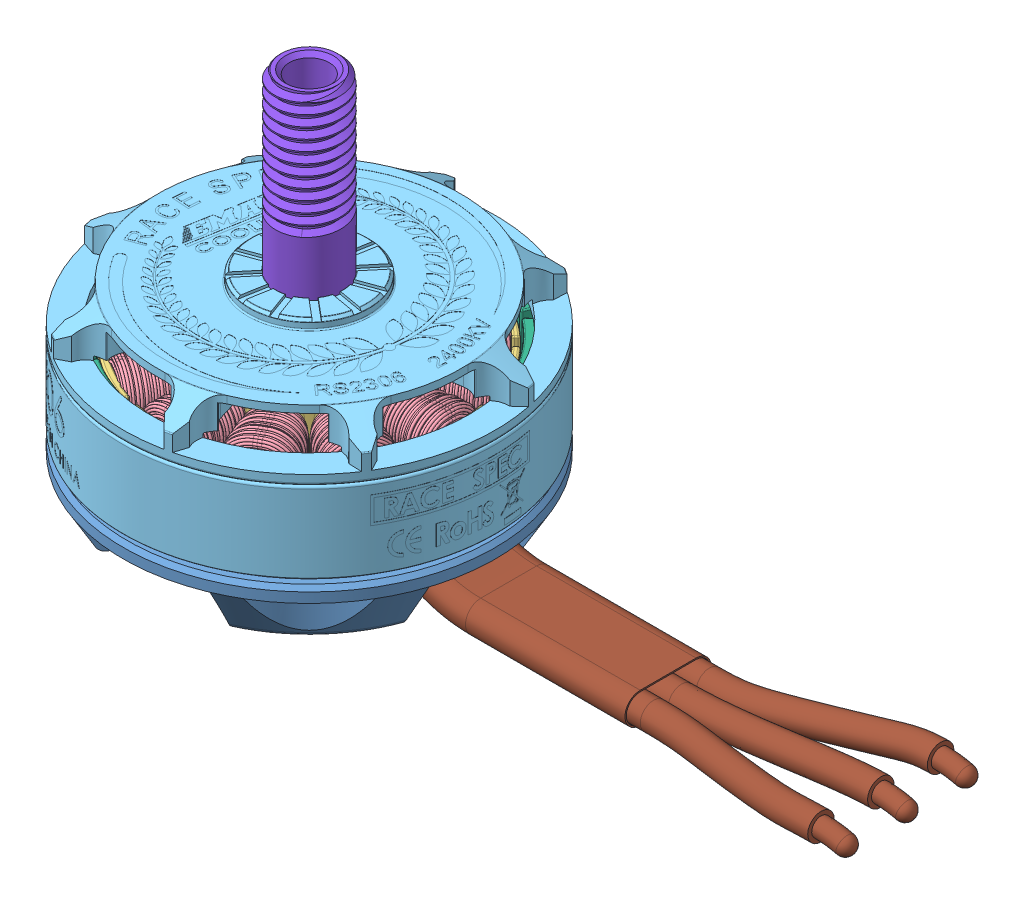
SolidWorks assembly EMAX RS2306, configuration Predeterminado. Lengths in mm.
Overall size (61.73 30.3 32.43).
25 component instances, 11 part files, 14 mates.
Components (placement in the parent):
- STATOR RS2306-1: STATOR RS2306 [Predeterminado] at origin size (28 11.98 28)
  - STATOR RS2306-1: STATOR RS2306 [Predeterminado] at origin size (28 10.77 28)
  - BEARING-1: BEARING [Predeterminado] at (0 2.25 0) x (1 0 0) z (0 1 0) size (8 8 3.5)
  - BEARING-2: BEARING [Predeterminado] at (0 8.85 0) x (-0.982082 0 -0.188455) z (0 -1 0) size (8 8 3.5)
  - STATOR SLEEVE-1: STATOR SLEEVE [Predeterminado] at (0 5.25 0) size (22.5 5.67 22.5)
  - WINDING-1: WINDING [Predeterminado] at (8.4112 8.075 0) size (4.68 7.47 4.47)
  - WINDING-2: WINDING [Predeterminado] at (7.2843 8.075 4.2056) x (0.866025 0 0.5) z (-0.5 0 0.866025) size (4.68 7.47 4.47)
  - WINDING-3: WINDING [Predeterminado] at (4.2056 8.075 7.2843) x (0.5 0 0.866025) z (-0.866025 0 0.5) size (4.68 7.47 4.47)
  - WINDING-4: WINDING [Predeterminado] at (0 8.075 8.4112) x (0 0 1) z (-1 0 0) size (4.68 7.47 4.47)
  - WINDING-5: WINDING [Predeterminado] at (-4.2056 8.075 7.2843) x (-0.5 0 0.866025) z (-0.866025 0 -0.5) size (4.68 7.47 4.47)
  - WINDING-6: WINDING [Predeterminado] at (-7.2843 8.075 4.2056) x (-0.866025 0 0.5) z (-0.5 0 -0.866025) size (4.68 7.47 4.47)
  - WINDING-7: WINDING [Predeterminado] at (-8.4112 8.075 0) x (-1 0 0) z (0 0 -1) size (4.68 7.47 4.47)
  - WINDING-8: WINDING [Predeterminado] at (-7.2843 8.075 -4.2056) x (-0.866025 0 -0.5) z (0.5 0 -0.866025) size (4.68 7.47 4.47)
  - WINDING-9: WINDING [Predeterminado] at (-4.2056 8.075 -7.2843) x (-0.5 0 -0.866025) z (0.866025 0 -0.5) size (4.68 7.47 4.47)
  - WINDING-10: WINDING [Predeterminado] at (0 8.075 -8.4112) x (0 0 -1) z (1 0 0) size (4.68 7.47 4.47)
  - WINDING-11: WINDING [Predeterminado] at (4.2056 8.075 -7.2843) x (0.5 0 -0.866025) z (0.866025 0 0.5) size (4.68 7.47 4.47)
  - WINDING-12: WINDING [Predeterminado] at (7.2843 8.075 -4.2056) x (0.866025 0 -0.5) z (0.5 0 0.866025) size (4.68 7.47 4.47)
- ROTOR RS2306-1: ROTOR RS2306 [Predeterminado] at (0 0.05 0) x (0.172455 0 -0.985017) z (0.985017 0 0.172455) size (28.01 28.45 28.01)
  - ROTOR BELL RS2306-1: ROTOR BELL RS2306 [Predeterminado] at origin size (28.01 10.2 28.01)
  - MAGNETS-1: MAGNETS [Predeterminado] at (0 5.3 0) size (25.73 6 25.8)
  - MAGNETS ADHESIVE-1: MAGNETS ADHESIVE [Predeterminado] at (0 5.4 0) size (26 5.9 26)
  - SHAFT RS2306-1: SHAFT RS2306 [Predeterminado] at (0 0.55 0) size (7.2 28.45 7.2)
- WASHER-1: WASHER [Predeterminado] at (0 -0.3 0) x (-0.985017 0 -0.172455) z (0.172455 0 -0.985017) size (5 0.8 5)
- SCREW-3: SCREW [ROSCADO] at (0 3.7 0) x (0 1 0) z (-0.466061 0 0.884753) size (5.25 3.8 3.8)
- MOTOR WIRES-1: MOTOR WIRES [Predeterminado] at (27 0.5 0) x (0 0 1) z (-1 0 0) size (11.02 5.68 38.85)
Mates (geometry in assembly coordinates):
- Coincidente1: coincident: plane of STATOR RS2306-1/STATOR RS2306-1 through (0 0 0) normal (0 0 1); plane of assembly through (0 0 0) normal (0 0 1)
- Coincidente2: coincident: plane of STATOR RS2306-1/STATOR RS2306-1 through (-11.2865 0 0) normal (0 -1 0); plane of assembly through (0 0 0) normal (0 1 0)
- Coincidente3: coincident: plane of STATOR RS2306-1/STATOR RS2306-1 through (0 0 0) normal (1 0 0); plane of assembly through (0 0 0) normal (1 0 0)
- Concéntrica1: concentric: cylinder of STATOR RS2306-1/STATOR RS2306-1 through (0 0 0) axis (0 -1 0) radius 14; cylinder of ROTOR RS2306-1/ROTOR BELL RS2306-1 through (0 0.05 0) axis (0 -1 0) radius 14
- Coincidente6: coincident: plane of STATOR RS2306-1/BEARING-2 through (0.3644 10.6 -1.8989) normal (0 1 0); plane of ROTOR RS2306-1/SHAFT RS2306-1 through (0.5001 10.6 -2.8566) normal (0 -1 0)
- Concéntrica2: concentric: cylinder of ROTOR RS2306-1/SHAFT RS2306-1 through (0 0.6 0) axis (0 -1 0) radius 0.8; cylinder of WASHER-1 through (0 0.5 0) axis (0 -1 0) radius 1.1
- Concéntrica41: concentric: cone of WASHER-1 through (0 -0.3 0) axis (0 1 0); cylinder of SCREW-3 through (0 3.7 0) axis (0 1 0) radius 1.9
- Coincidente91: coincident: plane of WASHER-1 through (0 -0.3 0) normal (0 -1 0); plane of SCREW-3 through (-0.9732 -0.3 -0.5127) normal (0 1 0)
- Bloquear1: lock: unknown of ?; unknown of SCREW-3
- Bloquear2: lock: unknown of ?; unknown of WASHER-1
- Coincidente93: coincident: plane of STATOR RS2306-1/BEARING-1 through (0 0.5 -1.9336) normal (0 -1 0); plane of WASHER-1 through (0 0.5 0) normal (0 1 0)
- Coincidente94: coincident: plane of MOTOR WIRES-1 through (27 0.5 0) normal (0 0 1); plane of assembly through (0 0 0) normal (0 0 1)
- Distancia1: distance = 0.5 mm: plane of MOTOR WIRES-1 through (27 0.5 -2.1) normal (0 1 0); plane of assembly through (0 0 0) normal (0 1 0)
- Distancia2: distance = 27 mm: plane of MOTOR WIRES-1 through (27 0.5 0) normal (-1 0 0); plane of assembly through (0 0 0) normal (1 0 0)
